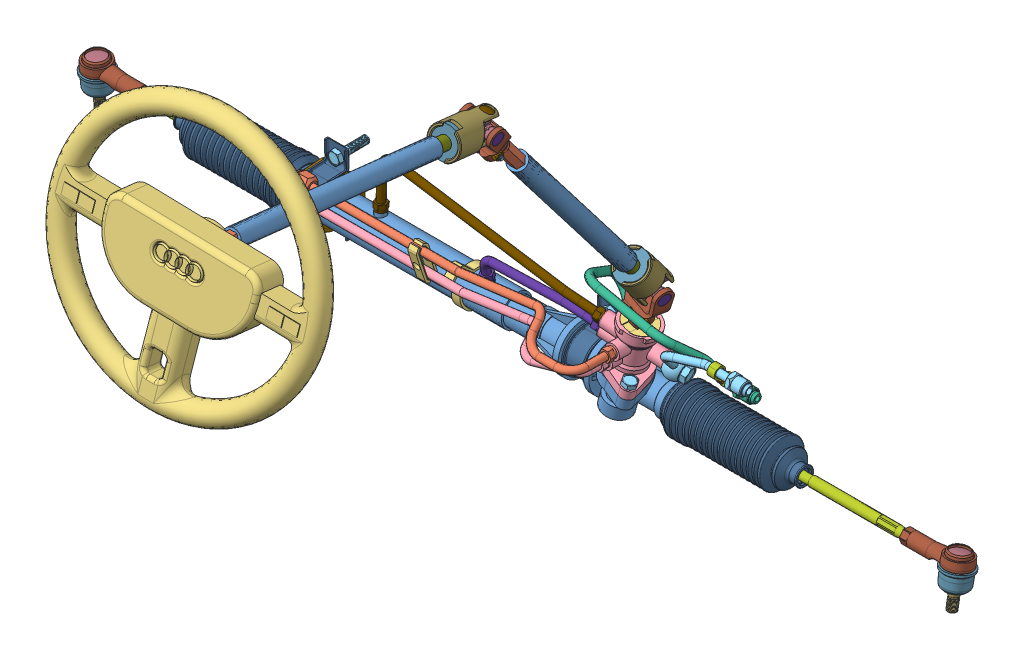
SolidWorks assembly 06, configuration Varsayılan. Lengths in mm.
Overall size (1248.7 876.17 925.76).
101 component instances, 57 part files, 133 mates.
Components (placement in the parent):
- 04-04-1: 04-04 [Varsayılan] at (-125.6681 -6.1583 231.0307) size (234.82 71.44 100.51)
- 04-02-1: 04-02 [Varsayılan] at (194.7465 -6.1583 231.0307) x (0 -1 0) z (-1 0 0) size (38 38 598)
- 04-03-1: 04-03 [Varsayılan] at (38.6922 -33.6461 251.0307) x (0.660997 -0.183782 0.727535) z (-0.700932 0.194939 0.686071) size (25.52 151.51 25.52)
- 04-01-1: 04-01 [Varsayılan] at (50.1654 -6.1583 196.9106) x (0 0 1) z (-1 0 0) size (4.12 38.49 38.49)
- 04-05-1: 04-05 [Varsayılan] at (50.1654 -6.1583 220.9669) x (0 0 1) z (-1 0 0) size (15.7 26.77 26.77)
- 04-06-1: 04-06 [Varsayılan] at (50.1654 -6.1583 203.9669) x (-1 0 0) z (0 0 -1) size (18.46 18.46 19.47)
- 04-07-1: 04-07 [Varsayılan] at (50.1654 -6.1583 223.256) x (0 0 1) z (-1 0 0) size (13.68 21.45 8.13)
- 04-08-1: 04-08 [Varsayılan] at (50.1654 -6.1583 218.4607) x (0 1 0) z (-1 0 0) size (28.57 26.12 28.57)
- 05-14-1: 05-14 [Varsayılan] at (37.0194 -39.6612 251.0307) x (0.963448 -0.267897 0) z (0 0 1) size (30.59 16.59 30.59)
- 05-15-1: 05-15 [Varsayılan] at (41.4642 -23.6793 251.0307) x (0.963434 -0.267944 0) z (0 0 1) size (27.84 7.6 27.84)
- 05-21-1: 05-21 [Varsayılan] at (38.6909 -33.6508 251.0307) x (0.928206 -0.258147 -0.267944) z (0.267944 0.963434 0) size (19.84 10.08 10.35)
- 05-09-1: 05-09 [Varsayılan] at (52.7201 16.7932 251.0307) x (0.963434 -0.267944 0) z (0 0 1) size (31.93 8.54 31.93)
- 05-24-1: 05-24 [Varsayılan] at (55.0081 25.02 251.0307) x (0.963434 -0.267944 0) z (0 0 1) size (34.48 1.46 34.48)
- 05-19-1: 05-19 [Varsayılan] at (66.8414 67.5685 251.0307) x (0.963434 -0.267944 0) z (0 0 1) size (24.62 1.21 24.62)
- 05-10-1: 05-10 [Varsayılan] at (57.7931 35.0339 251.0307) x (0.959223 -0.266824 -0.093253) z (0.089843 -0.024987 0.995642) size (34.48 33.93 34.48)
- 05-11-1: 05-11 [Varsayılan] at (60.4905 44.7327 251.0307) x (0.963421 -0.267991 0) z (0 0 1) size (34.47 2.04 34.47)
- 05-11-2: 05-11 [Varsayılan] at (62.3958 51.5835 251.0307) x (0.963421 -0.267991 0) z (0 0 1) size (34.47 2.04 34.47)
- 05-11-3: 05-11 [Varsayılan] at (64.317 58.4914 251.0307) x (0.963421 -0.267991 0) z (0 0 1) size (34.47 2.04 34.47)
- 05-11-4: 05-11 [Varsayılan] at (66.126 64.9963 251.0307) x (0.963421 -0.267991 0) z (0 0 1) size (34.47 2.04 34.47)
- 05-12-1: 05-12 [Varsayılan] at (67.6163 70.3549 251.0307) x (0.92973 -0.25852 0.26224) z (-0.252651 0.070266 0.965003) size (31.17 6.94 31.17)
- 05-13-1: 05-13 [Varsayılan] at (69.4753 77.0389 251.0307) x (0.963448 -0.267897 0) z (0 0 1) size (29.11 4.72 29.11)
- 05-16-1: 05-16 [Varsayılan] at (67.6164 70.3551 251.0307) x (0.963448 -0.267897 0) z (0 0 1) size (40.01 14.09 40.01)
- 05-22-3: 05-22 [Varsayılan] at (69.4711 77.0238 251.0307) x (0.963434 -0.267944 0) z (0 0 1) size (37.74 2.78 37.74)
- 05-18-1: 05-18 [Varsayılan] at (71.3908 83.9265 251.0307) x (0.96127 -0.267342 0.066993) z (-0.064543 0.01795 0.997753) size (40.8 2.9 40.8)
- 05-25-1: 05-25 [Varsayılan] at (57.2884 33.5525 251.0071) x (0.003637 -0.001047 -0.999993) z (0.963428 -0.267942 0.003784) size (68.03 67.23 77.18)
- formed hex screw_am-1: formed hex screw_am [B18.2.3.2M - Formed hex screw, M10 x 1.5 x 25 --25WS] at (82.3436 33.466 275.1353) x (-0.267944 -0.963434 0) z (0 0 1) size (31.63 18.48 16)
- formed hex screw_am-2: formed hex screw_am [B18.2.3.2M - Formed hex screw, M10 x 1.5 x 25 --25WS] at (36.0727 46.3346 226.9262) x (-0.267944 -0.963434 0) z (0 0 1) size (31.63 18.48 16)
- ROT MİLİ-1: ROT MİLİ [Varsayılan] at (-413.015 77.9473 255.0381) x (1 0 0) z (0 0.086009 -0.996294) size (284.47 41.76 37.89)
  - 02-02-2: 02-02 [Varsayılan] at (3.7615 85.8588 16.6847) size (48.52 36 36)
  - 02-03-3: 02-03 [Varsayılan] at (0.4735 85.8588 16.6847) x (-1 0 0) z (0 0.000479 1) size (257.66 24 24)
  - 02-01-2: 02-01 [Varsayılan] at (2.815 90.0301 15.9062) x (0.295289 -0.871295 0.391981) z (-0.068342 0.389963 0.918291) size (28 21.64 28)
- ROT MİLİ-2: ROT MİLİ [Varsayılan] at (204.5079 -67.283 293.5918) x (-1 0 0) z (0 -0.568825 -0.822459) size (284.47 41.76 37.89)
  - 02-02-2: 02-02 [Varsayılan] at (3.7615 85.8588 16.6847) size (48.52 36 36)
  - 02-03-3: 02-03 [Varsayılan] at (0.4735 85.8588 16.6847) x (-1 0 0) z (0 0.000479 1) size (257.66 24 24)
  - 02-01-2: 02-01 [Varsayılan] at (2.815 90.0301 15.9062) x (0.295289 -0.871295 0.391981) z (-0.068342 0.389963 0.918291) size (28 21.64 28)
- 05-31-1: 05-31 [Varsayılan] at (-390.0863 -6.1583 231.0307) x (0 0.999978 0.006566) z (0 0.006566 -0.999978) size (59.07 38.45 68.81)
- 05-02-1: 05-02 [Varsayılan] at (-409.0863 -6.1583 231.0307) x (-1 0 0) z (0 -0.999688 0.024965) size (174.75 66.11 66.11)
- 05-02-2: 05-02 [Varsayılan] at (105.6183 -6.1583 231.0307) size (174.75 66.11 66.11)
- ROT BAŞI-1: ROT BAŞI [Varsayılan] at (-663.7689 -10.787 321.1728) x (1 0 0) z (0 0.078367 -0.996925) size (99.29 68.51 54.56)
  - 03-01-1: 03-01 [Default] at (-37.7726 9.1069 90.2276) size (90.23 26.88 54.56)
  - 03-02-1: 03-02 [Varsayılan] at (-32.6694 53.6205 89.5242) x (0 -1 0) z (0.136534 0 0.990635) size (58.89 20 20)
  - 03-03-1: 03-03 [Varsayılan] at (-37.7726 -12.3176 90.2276) x (0.135044 0.003215 -0.990834) z (0.99084 0 0.135044) size (26.35 4.4 26.35)
  - 03-04-1: 03-04 [Varsayılan] at (-37.7726 28.686 90.2276) x (0.880691 0 -0.473691) z (0.473691 0 0.880691) size (39.96 25.57 39.96)
  - 03-05-1: 03-05 [Varsayılan] at (-37.7726 -9.866 90.2276) size (25.83 14.98 25.83)
- ROT BAŞI-2: ROT BAŞI [Varsayılan] at (455.2618 -18.6568 141.6394) x (-1 0 0) z (0 0.1653 0.986243) size (99.29 68.51 54.56)
  - 03-01-1: 03-01 [Default] at (-37.7726 9.1069 90.2276) size (90.23 26.88 54.56)
  - 03-02-1: 03-02 [Varsayılan] at (-32.6694 53.6205 89.5242) x (0 -1 0) z (0.136534 0 0.990635) size (58.89 20 20)
  - 03-03-1: 03-03 [Varsayılan] at (-37.7726 -12.3176 90.2276) x (0.135044 0.003215 -0.990834) z (0.99084 0 0.135044) size (26.35 4.4 26.35)
  - 03-04-1: 03-04 [Varsayılan] at (-37.7726 28.686 90.2276) x (0.880691 0 -0.473691) z (0.473691 0 0.880691) size (39.96 25.57 39.96)
  - 03-05-1: 03-05 [Varsayılan] at (-37.7726 -9.866 90.2276) size (25.83 14.98 25.83)
- 05-28-1: 05-28 [Varsayılan] at (-1.0263 -6.1583 231.0307) x (0 -0.759317 -0.650721) z (-1 0 0) size (54.92 54.94 38.56)
- 05-05-3: 05-05 [Varsayılan] at (-153.627 16.7021 236.5228) x (-0.999618 0.007048 -0.026719) z (0.027616 0.221471 -0.974776) size (188.63 111.65 20.5)
- 05-06-2: 05-06 [Varsayılan] at (-308.371 55.2453 229.576) x (-0.999565 0.002273 -0.029406) z (0.029339 -0.025305 -0.999249) size (348.36 140.05 41.18)
- 05-03-3: 05-03 [Varsayılan] at (-414.0863 -6.1583 231.0307) size (295 48.35 43.5)
- 05-33-1: 05-33 [Default] at (-156.8797 44.8002 297.1129) x (-1 0 0) z (0 0.302472 -0.953158) size (421.56 52.06 61.28)
- 05-01-1: 05-01 [Varsayılan] at (-173.5526 -6.1583 231.0307) x (-1 0 0) z (0 0.360562 -0.932735) size (14 137.7 76.92)
- 05-04-1: 05-04 [Varsayılan] at (-390.9146 51.2479 300.523) x (-0.991921 0.112405 0.058801) z (0.000453 0.46666 -0.884437) size (456.96 84.72 60.32)
- 05-08-1: 05-08 [Varsayılan] at (237.637 92.2948 265.4276) x (-0.997325 0.072053 -0.012308) z (-0.043043 -0.714977 -0.697822) size (140.05 46.48 89.04)
- 05-07-1: 05-07 [Varsayılan] at (228.5019 70.3353 246.6946) x (-0.999175 0.040461 0.003581) z (-0.026401 -0.579908 -0.814254) size (231 45.96 100.61)
- formed hex screw_am-3: formed hex screw_am [B18.2.3.2M - Formed hex screw, M12 x 1.75 x 25 --25WS] at (123.6594 37.5337 232.8376) x (-0.948079 0.263674 0.177825) z (-0.177825 -0.903067 0.390959) size (32.76 20.78 18)
- 05-27-1: 05-27 [Varsayılan] at (186.4406 76.9952 250.3773) x (0.044464 0.751851 0.657832) z (0.9987 -0.049876 -0.0105) size (45.68 8 10)
- 05-27-2: 05-27 [Varsayılan] at (196.4276 76.4964 250.2723) x (0.044464 0.751851 0.657832) z (-0.9987 0.049876 0.0105) size (45.68 8 10)
- hex screw_am-2: hex screw_am [B18.6.7M - M5 x 0.8 x 10 Indented HHMS --10S] at (191.9929 87.5632 252.0852) x (-0.024915 -0.657444 0.753091) z (-0.753091 0.507767 0.418362) size (13.8 9.24 8)
- prevailing torque hex nut_am-2: prevailing torque hex nut_am [AM-M5-S] at (191.6665 78.9507 261.9507) x (0.999646 -0.009344 0.024915) z (-0.024915 -0.657444 0.753091) size (8 9.81 5.3)
- 05-29-1: 05-29 [Default] at (-12.3188 -6.1583 205.6444) x (0 1 0) z (0 0 -1) size (108.96 30.28 55.85)
- 05-29-3: 05-29 [Default] at (-390.1285 -6.1115 206.1523) x (0 0.999914 0.013132) z (0 0.013132 -0.999914) size (108.96 30.28 55.85)
- formed hex screw_am-4: formed hex screw_am [B18.2.3.2M - Formed hex screw, M10 x 1.5 x 40 --26WS] at (-390.1268 33.0747 215.2976) x (0 0.013132 -0.999914) z (0.935126 0.354284 0.004653) size (46.63 18.48 16)
- formed hex screw_am-5: formed hex screw_am [B18.2.3.2M - Formed hex screw, M10 x 1.5 x 40 --26WS] at (-390.1268 -45.812 214.2616) x (0 0.013132 -0.999914) z (0.970956 -0.239236 -0.003142) size (46.63 18.48 16)
- formed hex screw_am-6: formed hex screw_am [B18.2.3.2M - Formed hex screw, M10 x 1.5 x 40 --26WS] at (-12.3171 -45.7489 214.2744) x (0 0 -1) z (0.991782 -0.12794 0) size (46.63 18.48 16)
- formed hex screw_am-7: formed hex screw_am [B18.2.3.2M - Formed hex screw, M10 x 1.5 x 40 --26WS] at (-12.3171 33.1445 213.7744) x (0 0 -1) z (0.999706 0.024251 0) size (46.63 18.48 16)
- UNIVERSAL MAFSAL-1: UNIVERSAL MAFSAL [Varsayılan] at (141.0332 165.171 256.4603) x (0.950533 -0.264356 0.163103) z (-0.267944 -0.963434 0) size (48.16 92.97 129.43)
  - 01-01-1: 01-01 [Varsayılan] at (-45.6055 2.036 86.4549) size (47 34.99 57.64)
  - 01-02-1: 01-02 [Varsayılan] at (-45.0363 8.2494 31.8587) x (-0.051046 -0.624854 0.779071) z (0 -0.780088 -0.62567) size (70.3 43.23 43.34)
  - 01-03-1: 01-03 [Varsayılan] at (-51.6055 -0.2661 32.8861) x (1 0 0) z (0 -0.62567 0.780088) size (36 31 16)
  - 01-04-1: 01-04 [Varsayılan] at (-42.5986 38.09 -5.3467) x (-0.998696 0.031938 -0.03982) z (-0.051046 -0.624854 0.779071) size (33.8 41.3 6)
  - 01-05-1: 01-05 [Varsayılan] at (-42.9049 34.3409 -0.6723) x (0.998255 -0.008733 0.058403) z (0.02969 -0.780692 -0.62421) size (32.2 29.4 32.2)
  - 01-06-1: 01-06 [Varsayılan] at (-44.4056 15.9701 22.2324) x (0.051046 0.624854 -0.779071) z (0.993628 0.046715 0.102572) size (75.7 17.29 17.32)
  - 01-07-1: 01-07 [Varsayılan] at (-25.3055 1.2861 40.5406) x (0 0 -1) z (1 0 0) size (16 16 15)
  - 01-08-1: 01-08 [Varsayılan] at (-45.6055 -12.5995 29.4036) x (0.792707 0.38141 -0.475544) z (0 -0.780088 -0.62567) size (16 16 15)
  - 01-07-2: 01-07 [Varsayılan] at (-65.9055 1.2861 40.5406) x (0 -0.633294 0.773912) z (-1 0 0) size (16 16 15)
  - 01-08-2: 01-08 [Varsayılan] at (-45.6055 15.1716 51.6775) x (0.990366 0.086641 -0.108024) z (0 0.780088 0.62567) size (16 16 15)
  - formed hex screw_am-1: formed hex screw_am [B18.2.3.2M - Formed hex screw, M6 x 1.0 x 35 --18WS] at (-62.5055 12.536 76.9549) x (1 0 0) z (0 0.052048 -0.998645) size (39.15 11.55 10)
  - prevailing torque hex nut_am-1: prevailing torque hex nut_am [AM-M6-S] at (-26.1555 12.536 76.9549) x (0 0.889289 0.457347) z (1 0 0) size (10.79 11.55 6.7)
- SHAFT 1-1: SHAFT 1 [Varsayılan] at (102.4 214.0531 312.2723) x (0.979633 -0.04367 -0.195992) z (0.15908 0.764397 0.624813) size (24 24 322.5)
- SHAFT 2-1: SHAFT 2 [Varsayılan] at (126.2619 328.7127 405.9942) x (-0.986743 0.10251 0.125818) z (0.15908 0.764397 0.624813) size (19 19 232)
- UNIVERSAL MAFSAL-2: UNIVERSAL MAFSAL [Varsayılan] at (218.869 550.0843 590.8605) x (0.981176 -0.192592 -0.014194) z (-0.15908 -0.764397 -0.624813) size (48.16 92.97 129.43)
  - 01-01-1: 01-01 [Varsayılan] at (-45.6055 2.036 86.4549) size (47 34.99 57.64)
  - 01-02-1: 01-02 [Varsayılan] at (-45.0363 8.2494 31.8587) x (-0.051046 -0.624854 0.779071) z (0 -0.780088 -0.62567) size (70.3 43.23 43.34)
  - 01-03-1: 01-03 [Varsayılan] at (-51.6055 -0.2661 32.8861) x (1 0 0) z (0 -0.62567 0.780088) size (36 31 16)
  - 01-04-1: 01-04 [Varsayılan] at (-42.5986 38.09 -5.3467) x (-0.998696 0.031938 -0.03982) z (-0.051046 -0.624854 0.779071) size (33.8 41.3 6)
  - 01-05-1: 01-05 [Varsayılan] at (-42.9049 34.3409 -0.6723) x (0.998255 -0.008733 0.058403) z (0.02969 -0.780692 -0.62421) size (32.2 29.4 32.2)
  - 01-06-1: 01-06 [Varsayılan] at (-44.4056 15.9701 22.2324) x (0.051046 0.624854 -0.779071) z (0.993628 0.046715 0.102572) size (75.7 17.29 17.32)
  - 01-07-1: 01-07 [Varsayılan] at (-25.3055 1.2861 40.5406) x (0 0 -1) z (1 0 0) size (16 16 15)
  - 01-08-1: 01-08 [Varsayılan] at (-45.6055 -12.5995 29.4036) x (0.792707 0.38141 -0.475544) z (0 -0.780088 -0.62567) size (16 16 15)
  - 01-07-2: 01-07 [Varsayılan] at (-65.9055 1.2861 40.5406) x (0 -0.633294 0.773912) z (-1 0 0) size (16 16 15)
  - 01-08-2: 01-08 [Varsayılan] at (-45.6055 15.1716 51.6775) x (0.990366 0.086641 -0.108024) z (0 0.780088 0.62567) size (16 16 15)
  - formed hex screw_am-1: formed hex screw_am [B18.2.3.2M - Formed hex screw, M6 x 1.0 x 35 --18WS] at (-62.5055 12.536 76.9549) x (1 0 0) z (0 0.052048 -0.998645) size (39.15 11.55 10)
  - prevailing torque hex nut_am-1: prevailing torque hex nut_am [AM-M6-S] at (-26.1555 12.536 76.9549) x (0 0.889289 0.457347) z (1 0 0) size (10.79 11.55 6.7)
- SHAFT 1-2: SHAFT 1 [Varsayılan] at (178.0086 547.047 663.7863) x (0.966904 0.207955 -0.147823) z (0.105608 0.201209 0.973839) size (24 24 322.5)
- SHAFT 2-2: SHAFT 2 [Varsayılan] at (191.7377 573.2042 790.3853) x (-0.99018 0.111484 0.084346) z (0.105608 0.201209 0.973839) size (19 19 232)
- direksiyon-1: direksiyon [Varsayılan] at (216.7667 620.8908 1021.1848) x (-0.99018 0.111484 0.084346) z (0.105608 0.201209 0.973839) size (350 350 50.57)
Mates (geometry in assembly coordinates):
- Eş Merkezli1: concentric aligned: cylinder of 04-04-1 through (-165.266 -6.1583 231.0307) axis (1 0 0) radius 14; cylinder of 04-02-1 through (-403.2535 -6.1583 231.0307) axis (1 0 0) radius 11.5
- Eş Merkezli2: concentric anti-aligned: cylinder of 04-04-1 through (54.1024 21.7633 251.0307) axis (0.267944 0.963434 0) radius 12.4576; line of 04-03-1 through (79.2895 112.3275 251.0307) axis (-0.267944 -0.963434 0)
- Teğet1: tangent aligned: plane of 04-04-1 through (55.5026 -19.6951 251.0307) normal (-0.267944 -0.963434 0); cone of 04-03-1 through (43.5006 -16.3571 251.0307) axis (-0.267944 -0.963434 0)
- Paralel1: parallel: plane of 04-02-1 through (31.8195 10.9835 238.0307) normal (0 0 1); line of 04-03-1 through (79.2895 112.3275 251.0307) axis (-0.267944 -0.963434 0)
- RackPinionMate1: rack pinion = 20 mm: line of 04-02-1 through (-6.8954 -15.2825 238.0307) axis (-1 0 0); circle of 04-03-1
- Uzaklığı Sınırla1: limit distance = 59.5855 mm anti-aligned: plane of 04-04-1 through (-125.6681 11.3406 231.0307) normal (-1 0 0); plane of 04-02-1 through (-185.2535 -6.1583 250.0307) normal (1 0 0)
- Eş Merkezli3: concentric anti-aligned: cylinder of 04-05-1 through (50.1654 -6.1583 220.9669) axis (0 0 -1) radius 3.705; cylinder of 04-07-1 through (50.1654 -6.1583 223.256) axis (0 0 1) radius 3.7071
- Eş Merkezli4: concentric: sphere of 04-05-1; sphere of 04-07-1
- Eş Merkezli5: concentric anti-aligned: circle of 04-06-1; cylinder of 04-07-1 through (50.1654 -6.1583 223.256) axis (0 0 1) radius 3.7071
- Çakışık1: coincident anti-aligned: plane of 04-05-1 through (59.8031 -6.1583 220.9669) normal (0 0 -1); plane of 04-06-1 through (40.4527 -15.387 220.9669) normal (0 0 1)
- Eş Merkezli6: concentric anti-aligned: circle of 04-06-1; cylinder of 04-08-1 through (50.1654 -6.1583 199.3607) axis (0 0 1) radius 14.285
- Çakışık2: coincident anti-aligned: plane of 04-05-1 through (63.3694 -6.1583 218.4607) normal (0 0 -1); plane of 04-08-1 through (50.1654 -6.1583 218.4607) normal (0 0 1)
- Eş Merkezli7: concentric anti-aligned: cylinder of 04-04-1 through (50.1654 -6.1583 285.0814) axis (0 0 -1) radius 14; cylinder of 04-08-1 through (50.1654 -6.1583 199.3607) axis (0 0 1) radius 14.285
- Çakışık3: coincident anti-aligned: plane of 04-04-1 through (50.1654 -6.1583 201.0307) normal (0 0 -1); circle of 04-08-1
- Eş Merkezli8: concentric anti-aligned: cylinder of 04-04-1 through (50.1654 -6.1583 201.0307) axis (0 0 1) radius 18.85; cylinder of 04-01-1 through (50.1654 -6.1583 196.9106) axis (0 0 -1) radius 13.3852
- Çakışık4: coincident anti-aligned: plane of 04-04-1 through (50.1654 -6.1583 201.0307) normal (0 0 -1); plane of 04-01-1 through (63.5506 -6.1583 201.0307) normal (0 0 1)
- Eş Merkezli9: concentric anti-aligned: cylinder of 04-04-1 through (54.1024 21.7633 251.0307) axis (0.267944 0.963434 0) radius 15.0252; cylinder of 05-15-1 through (43.5005 -16.3572 251.0307) axis (-0.267944 -0.963434 0) radius 13.92
- Çakışık5: coincident anti-aligned: plane of 04-04-1 through (55.5026 -19.6951 251.0307) normal (-0.267944 -0.963434 0); plane of 05-15-1 through (43.5005 -16.3572 251.0307) normal (0.267944 0.963434 0)
- Eş Merkezli10: concentric aligned: cone of 04-03-1 through (38.6923 -33.6459 251.0307) axis (0.267944 0.963434 0); cylinder of 05-21-1 through (38.6909 -33.6508 251.0307) axis (0.267944 0.963434 0) radius 4.26
- Çakışık6: coincident anti-aligned: plane of 05-15-1 through (41.4642 -23.6793 251.0307) normal (-0.267944 -0.963434 0); plane of 05-21-1 through (41.4642 -23.6793 251.0307) normal (0.267944 0.963434 0)
- Eş Merkezli11: concentric aligned: cylinder of 04-04-1 through (54.1024 21.7633 251.0307) axis (0.267944 0.963434 0) radius 15.0252; cone of 05-14-1 through (39.1828 -31.8821 251.0307) axis (0.267944 0.963434 0)
- Teğet2: tangent aligned: cone of 05-14-1 through (41.4644 -23.6786 251.0307) axis (-0.267944 -0.963434 0); plane of 05-15-1 through (41.4642 -23.6793 251.0307) normal (-0.267944 -0.963434 0)
- Çakışık7: coincident: circle of 04-03-1; cone of 05-09-1 through (52.7203 16.7938 251.0307) axis (-0.267944 -0.963434 0)
- Eş Merkezli13: concentric anti-aligned: cylinder of 04-03-1 through (38.6922 -33.6461 251.0307) axis (-0.267944 -0.963434 0) radius 12.7592; cone of 05-24-1 through (55.3984 26.4235 251.0307) axis (0.267944 0.963434 0)
- Çakışık8: coincident aligned: cone of 05-09-1 through (55.008 25.0198 251.0307) axis (-0.267944 -0.963434 0); cone of 05-24-1 through (55.0081 25.02 251.0307) axis (-0.267944 -0.963434 0)
- Eş Merkezli14: concentric anti-aligned: cone of 04-03-1 through (67.1664 68.737 251.0307) axis (0.267944 0.963434 0); circle of 05-19-1
- Teğet4: tangent aligned: cone of 04-03-1 through (66.8415 67.569 251.0307) axis (-0.267944 -0.963434 0); plane of 05-19-1 through (66.8414 67.5685 251.0307) normal (-0.267944 -0.963434 0)
- Eş Merkezli15: concentric anti-aligned: cone of 04-03-1 through (67.1664 68.737 251.0307) axis (0.267944 0.963434 0); cone of 05-10-1 through (58.0414 35.9269 251.0307) axis (-0.267944 -0.963434 0)
- Teğet5: tangent aligned: plane of 05-19-1 through (66.8414 67.5685 251.0307) normal (-0.267944 -0.963434 0); cone of 05-10-1 through (66.8415 67.569 251.0307) axis (-0.267944 -0.963434 0)
- Eş Merkezli17: concentric aligned: cone of 05-10-1 through (60.4905 44.7327 251.0307) axis (0.267944 0.963434 0); cone of 05-11-1 through (61.036 46.6943 251.0307) axis (0.267944 0.963434 0)
- Çakışık10: coincident: circle of 05-10-1; cone of 05-11-1 through (60.4905 44.7327 251.0307) axis (-0.267944 -0.963434 0)
- Eş Merkezli18: concentric aligned: cone of 05-10-1 through (62.3958 51.5835 251.0307) axis (0.267944 0.963434 0); cone of 05-11-2 through (62.9413 53.5452 251.0307) axis (0.267944 0.963434 0)
- Çakışık11: coincident: circle of 05-10-1; cone of 05-11-2 through (62.3958 51.5835 251.0307) axis (-0.267944 -0.963434 0)
- Eş Merkezli19: concentric aligned: cone of 05-10-1 through (64.317 58.4914 251.0307) axis (0.267944 0.963434 0); cone of 05-11-3 through (64.8625 60.4531 251.0307) axis (0.267944 0.963434 0)
- Çakışık12: coincident: circle of 05-10-1; cone of 05-11-3 through (64.317 58.4914 251.0307) axis (-0.267944 -0.963434 0)
- Eş Merkezli20: concentric aligned: cone of 05-10-1 through (66.126 64.9963 251.0307) axis (0.267944 0.963434 0); cone of 05-11-4 through (66.6716 66.9579 251.0307) axis (0.267944 0.963434 0)
- Çakışık13: coincident: circle of 05-10-1; cone of 05-11-4 through (66.126 64.9963 251.0307) axis (-0.267944 -0.963434 0)
- Eş Merkezli22: concentric aligned: cone of 04-03-1 through (67.1664 68.737 251.0307) axis (0.267944 0.963434 0); cone of 05-12-1 through (69.4753 77.0389 251.0307) axis (0.267944 0.963434 0)
- Uzaklık1: distance = 2.73 mm aligned: cone of 05-12-1 through (67.6163 70.3549 251.0307) axis (-0.267944 -0.963434 0); cone of 05-10-1 through (66.8849 67.725 251.0307) axis (-0.267944 -0.963434 0)
- Eş Merkezli23: concentric aligned: cone of 04-03-1 through (67.1664 68.737 251.0307) axis (0.267944 0.963434 0); cone of 05-13-1 through (70.7393 81.5839 251.0307) axis (0.267944 0.963434 0)
- Çakışık14: coincident aligned: cone of 05-12-1 through (69.4753 77.0392 251.0307) axis (-0.267944 -0.963434 0); cone of 05-13-1 through (69.4753 77.0389 251.0307) axis (-0.267944 -0.963434 0)
- Eş Merkezli24: concentric aligned: cone of 05-12-1 through (67.6164 70.3551 251.0307) axis (0.267944 0.963434 0); cone of 05-16-1 through (67.6165 70.3553 251.0307) axis (0.267944 0.963434 0)
- Çakışık15: coincident aligned: cone of 05-12-1 through (67.6163 70.3549 251.0307) axis (-0.267944 -0.963434 0); cone of 05-16-1 through (67.6164 70.3551 251.0307) axis (-0.267944 -0.963434 0)
- Eş Merkezli25: concentric anti-aligned: cone of 05-16-1 through (69.4711 77.0238 251.0307) axis (0.267944 0.963434 0); cylinder of 05-22-3 through (70.216 79.7022 251.0307) axis (-0.267944 -0.963434 0) radius 18.87
- Çakışık16: coincident aligned: circle of 05-16-1; plane of 05-22-3 through (69.4711 77.0238 251.0307) normal (-0.267944 -0.963434 0)
- Eş Merkezli26: concentric anti-aligned: cone of 04-03-1 through (67.1664 68.737 251.0307) axis (0.267944 0.963434 0); cylinder of 05-18-1 through (76.4549 102.1354 251.0307) axis (-0.267944 -0.963434 0) radius 9.8
- Teğet6: tangent aligned: cone of 05-16-1 through (71.391 83.9274 251.0307) axis (-0.267944 -0.963434 0); plane of 05-18-1 through (71.3908 83.9265 251.0307) normal (-0.267944 -0.963434 0)
- Eş Merkezli27: concentric aligned: cylinder of 04-04-1 through (47.6487 -91.2848 275.1353) axis (0.267944 0.963434 0) radius 5.0797; cylinder of 05-25-1 through (77.2955 15.3149 275.1353) axis (0.267944 0.963434 0) radius 4.95
- Eş Merkezli28: concentric aligned: cylinder of 04-04-1 through (1.3778 -78.4162 226.9262) axis (0.267944 0.963434 0) radius 4.95; cylinder of 05-25-1 through (31.0246 28.1834 226.9262) axis (0.267944 0.963434 0) radius 5.0797
- Çakışık17: coincident anti-aligned: plane of 04-04-1 through (81.3463 14.1883 251.0307) normal (0.267944 0.963434 0); plane of 05-25-1 through (54.0168 21.789 251.0071) normal (-0.267944 -0.963434 0)
- Eş Merkezli291: concentric aligned: cylinder of 05-25-1 through (77.2955 15.3149 275.1353) axis (0.267944 0.963434 0) radius 4.95; cylinder of formed hex screw_am-1 through (82.3436 33.466 275.1353) axis (0.267944 0.963434 0) radius 5
- Çakışık181: coincident anti-aligned: plane of 05-25-1 through (57.2884 33.5525 251.0071) normal (0.267944 0.963434 0); plane of formed hex screw_am-1 through (89.4669 24.6032 275.1353) normal (-0.267944 -0.963434 0)
- Eş Merkezli301: concentric aligned: cylinder of 05-25-1 through (31.0246 28.1834 226.9262) axis (0.267944 0.963434 0) radius 5.0797; cylinder of formed hex screw_am-2 through (36.0727 46.3346 226.9262) axis (0.267944 0.963434 0) radius 5
- Çakışık191: coincident anti-aligned: plane of 05-25-1 through (57.2884 33.5525 251.0071) normal (0.267944 0.963434 0); plane of formed hex screw_am-2 through (43.196 37.4718 226.9262) normal (-0.267944 -0.963434 0)
- Eş Merkezli32: concentric anti-aligned: cylinder of 04-02-1 through (-403.2535 -6.1583 231.0307) axis (1 0 0) radius 11.5; cylinder of ROT MİLİ-1/02-02-2 through (-409.407 -6.1583 231.0307) axis (-1 0 0) radius 18
- Çakışık20: coincident anti-aligned: plane of 04-02-1 through (-403.2535 -6.1583 231.0307) normal (-1 0 0); plane of ROT MİLİ-1/02-02-2 through (-403.2535 -6.1583 231.0307) normal (1 0 0)
- Eş Merkezli33: concentric aligned: cylinder of 04-02-1 through (-403.2535 -6.1583 231.0307) axis (1 0 0) radius 11.5; cylinder of ROT MİLİ-2/02-02-2 through (200.8999 -6.1583 231.0307) axis (1 0 0) radius 18
- Çakışık21: coincident anti-aligned: plane of 04-02-1 through (194.7465 -6.1583 231.0307) normal (1 0 0); plane of ROT MİLİ-2/02-02-2 through (194.7465 -6.1583 231.0307) normal (-1 0 0)
- Eş Merkezli36: concentric anti-aligned: cylinder of 04-02-1 through (-403.2535 -6.1583 231.0307) axis (1 0 0) radius 11.5; cylinder of 05-02-2 through (105.6183 -6.1583 231.0307) axis (-1 0 0) radius 11.6806
- Çakışık23: coincident anti-aligned: plane of 04-04-1 through (105.6183 12.6764 231.0307) normal (1 0 0); plane of 05-02-2 through (105.6183 19.7754 231.0307) normal (-1 0 0)
- Eş Merkezli37: concentric aligned: cylinder of ROT MİLİ-1/02-03-3 through (-423.5415 -6.1583 231.0307) axis (1 0 0) radius 5.0675; cylinder of ROT BAŞI-1/03-01-1 through (-666.2915 -6.1583 231.0307) axis (1 0 0) radius 9.5
- Çakışık24: coincident aligned: circle of ROT MİLİ-1/02-03-3; plane of ROT BAŞI-1/03-01-1 through (-629.5415 3.069 222.1124) normal (1 0 0)
- Eş Merkezli38: concentric aligned: cylinder of ROT MİLİ-2/02-03-3 through (215.0344 -6.1583 231.0307) axis (-1 0 0) radius 6.5; cylinder of ROT BAŞI-2/03-01-1 through (457.7844 -6.1583 231.0307) axis (-1 0 0) radius 9.5
- Çakışık25: coincident aligned: circle of ROT MİLİ-2/02-03-3; plane of ROT BAŞI-2/03-01-1 through (421.0344 3.8139 239.1074) normal (-1 0 0)
- Eş Merkezli39: concentric anti-aligned: cylinder of 04-04-1 through (-125.6681 -6.1583 231.0307) axis (-1 0 0) radius 21.75; cylinder of 05-28-1 through (-23.5863 -6.1583 231.0307) axis (1 0 0) radius 25.75
- Çakışık26: coincident anti-aligned: plane of 04-04-1 through (6.9737 26.3417 231.0307) normal (-1 0 0); plane of 05-28-1 through (6.9737 -6.1583 231.0307) normal (1 0 0)
- Eş Merkezli304: concentric anti-aligned: cylinder of 05-25-1 through (101.3768 36.6462 241.4658) axis (-0.949417 0.264046 0.169963) radius 5; cylinder of 05-05-3 through (21.6687 58.8141 255.7351) axis (0.949417 -0.264046 -0.169963) radius 7
- Çakışık194: coincident anti-aligned: plane of 05-25-1 through (21.5918 48.3269 253.9468) normal (-0.949417 0.264046 0.169963); plane of 05-05-3 through (26.0012 62.678 256.2827) normal (0.949417 -0.264046 -0.169963)
- Eş Merkezli305: concentric anti-aligned: cylinder of 05-25-1 through (105.7565 50.9201 243.7559) axis (-0.949417 0.264046 0.169963) radius 5; cylinder of 05-06-2 through (26.0484 73.088 258.0251) axis (0.949417 -0.264046 -0.169963) radius 7
- Çakışık195: coincident anti-aligned: plane of 05-25-1 through (21.5918 48.3269 253.9468) normal (-0.949417 0.264046 0.169963); plane of 05-06-2 through (30.1982 77.1184 257.2936) normal (0.949417 -0.264046 -0.169963)
- Eş Merkezli306: concentric anti-aligned: cylinder of 04-02-1 through (-403.2535 -6.1583 231.0307) axis (1 0 0) radius 11.5; cylinder of 05-03-3 through (-119.0863 -6.1583 231.0307) axis (-1 0 0) radius 21.75
- Çakışık196: coincident anti-aligned: plane of 04-04-1 through (-119.0863 12.8417 231.0307) normal (-1 0 0); plane of 05-03-3 through (-119.0863 -6.1583 231.0307) normal (1 0 0)
- Eş Merkezli307: concentric anti-aligned: cylinder of 05-31-1 through (-405.0863 -6.1583 231.0307) axis (1 0 0) radius 20.7084; cylinder of 05-03-3 through (-119.0863 -6.1583 231.0307) axis (-1 0 0) radius 21.75
- Eş Merkezli308: concentric anti-aligned: cylinder of 05-02-1 through (-409.0863 -6.1583 231.0307) axis (1 0 0) radius 25.6827; cylinder of 05-03-3 through (-119.0863 -6.1583 231.0307) axis (-1 0 0) radius 21.75
- Uzaklık2: distance = 5 mm aligned: plane of 05-03-3 through (-414.0863 -6.1583 231.0307) normal (-1 0 0); plane of 05-31-1 through (-409.0863 -6.1583 231.0307) normal (-1 0 0)
- Çakışık197: coincident anti-aligned: plane of 05-31-1 through (-409.0863 -6.1583 231.0307) normal (-1 0 0); plane of 05-02-1 through (-409.0863 -6.8058 205.105) normal (1 0 0)
- Kilitle1: lock: unknown of 05-05-3; unknown of 05-03-3
- Kilitle2: lock: unknown of 05-06-2; unknown of 05-03-3
- Eş Merkezli309: concentric anti-aligned: cylinder of 05-25-1 through (65.5394 62.2675 263.2963) axis (-0.003655 0.006527 0.999972) radius 5; cylinder of 05-33-1 through (65.3201 62.6591 323.2946) axis (0.003655 -0.006527 -0.999972) radius 4
- Çakışık198: coincident anti-aligned: plane of 05-25-1 through (60.6154 54.5186 283.3295) normal (-0.003655 0.006527 0.999972); plane of 05-33-1 through (65.4663 62.3981 283.2958) normal (0.003655 -0.006527 -0.999972)
- Eş Merkezli310: concentric anti-aligned: cylinder of 05-03-3 through (-119.0863 -6.1583 231.0307) axis (-1 0 0) radius 21.75; cylinder of 05-01-1 through (-185.5526 -6.1583 231.0307) axis (1 0 0) radius 21.7671
- Teğet7: tangent anti-aligned: cylinder of 05-33-1 through (-125.1716 75.9211 306.9887) axis (-1 0 0) radius 5; plane of 05-01-1 through (-172.5526 79.1244 302.774) normal (0 -0.309917 0.950763)
- Eş Merkezli312: concentric anti-aligned: cylinder of 05-25-1 through (55.8376 46.5086 263.3637) axis (-0.003655 0.006527 0.999972) radius 5; circle of 05-04-1
- Çakışık201: coincident anti-aligned: plane of 05-25-1 through (60.6154 54.5186 283.3295) normal (-0.003655 0.006527 0.999972); plane of 05-04-1 through (60.0822 49.1995 283.3622) normal (0.003655 -0.006527 -0.999972)
- Kilitle3: lock: unknown of 05-01-1; unknown of 05-04-1
- Eş Merkezli313: concentric aligned: cylinder of 05-25-1 through (18.9204 66.663 252.4828) axis (0.948079 -0.263674 -0.177825) radius 5; cylinder of 05-08-1 through (83.9328 48.5821 240.2888) axis (0.948079 -0.263674 -0.177825) radius 5
- Çakışık202: coincident anti-aligned: plane of 05-25-1 through (97.3407 44.8532 237.774) normal (0.948079 -0.263674 -0.177825); plane of 05-08-1 through (101.3663 42.9237 262.0976) normal (-0.948079 0.263674 0.177825)
- Eş Merkezli314: concentric anti-aligned: cylinder of 05-25-1 through (91.8203 46.3885 292.2446) axis (-0.66663 0.185399 -0.721963) radius 5; cylinder of 05-07-1 through (28.8333 63.9061 224.0295) axis (0.66663 -0.185399 0.721963) radius 3
- Çakışık203: coincident anti-aligned: plane of 05-25-1 through (40.3095 60.7144 222.006) normal (-0.66663 0.185399 -0.721963); plane of 05-07-1 through (29.8159 63.3842 232.381) normal (0.66663 -0.185399 0.721963)
- Eş Merkezli3151: concentric aligned: cylinder of 05-08-1 through (83.9328 48.5821 240.2888) axis (0.948079 -0.263674 -0.177825) radius 5; cylinder of formed hex screw_am-3 through (123.6594 37.5337 232.8376) axis (0.948079 -0.263674 -0.177825) radius 6
- Çakışık2041: coincident anti-aligned: plane of 05-08-1 through (120.4882 37.9933 258.8874) normal (0.948079 -0.263674 -0.177825); plane of formed hex screw_am-3 through (113.5621 36.0564 224.8326) normal (-0.948079 0.263674 0.177825)
- Eş Merkezli316: concentric anti-aligned: cylinder of 05-08-1 through (180.9639 95.1251 266.0234) axis (0.9987 -0.049876 -0.0105) radius 5; cylinder of 05-27-1 through (197.4805 94.3003 265.8497) axis (-0.9987 0.049876 0.0105) radius 8
- Kilitle4: lock: unknown of 05-07-1; unknown of 05-27-1
- Eş Merkezli320: concentric anti-aligned: cylinder of 05-27-1 through (191.5494 75.8607 265.4902) axis (0.024915 0.657444 -0.753091) radius 2.5; cylinder of 05-27-2 through (192.1473 91.6394 247.416) axis (-0.024915 -0.657444 0.753091) radius 2.5
- Çakışık206: coincident anti-aligned: plane of 05-27-1 through (196.4276 76.4964 250.2723) normal (0.024915 0.657444 -0.753091); plane of 05-27-2 through (186.4406 76.9952 250.3773) normal (-0.024915 -0.657444 0.753091)
- Paralel2: parallel aligned: plane of 05-27-1 through (196.1608 71.9853 246.3253) normal (0.9987 -0.049876 -0.0105); plane of 05-27-2 through (196.1608 71.9853 246.3253) normal (0.9987 -0.049876 -0.0105)
- Eş Merkezli3221: concentric anti-aligned: cylinder of 05-27-2 through (192.1473 91.6394 247.416) axis (-0.024915 -0.657444 0.753091) radius 2.5; cylinder of hex screw_am-2 through (192.6257 104.2623 232.9567) axis (0.024915 0.657444 -0.753091) radius 2.5
- Çakışık2091: coincident anti-aligned: plane of 05-27-2 through (187.1989 90.2901 259.353) normal (0.024915 0.657444 -0.753091); plane of hex screw_am-2 through (193.5418 86.4567 256.2164) normal (-0.024915 -0.657444 0.753091)
- Eş Merkezli3231: concentric anti-aligned: cylinder of 05-27-1 through (191.5494 75.8607 265.4902) axis (0.024915 0.657444 -0.753091) radius 2.5; cylinder of prevailing torque hex nut_am-2 through (192.2903 95.4115 243.0952) axis (-0.024915 -0.657444 0.753091) radius 2.5
- Çakışık2101: coincident anti-aligned: plane of 05-27-1 through (197.0863 87.1616 262.2604) normal (-0.024915 -0.657444 0.753091); plane of prevailing torque hex nut_am-2 through (191.7554 85.9152 260.9959) normal (0.024915 0.657444 -0.753091)
- Eş Merkezli324: concentric anti-aligned: cylinder of 05-28-1 through (-23.5863 -6.1583 231.0307) axis (1 0 0) radius 25.75; circle of 05-29-1
- Paralel3: parallel aligned: plane of 04-08-1 through (50.1654 -6.1583 192.3407) normal (0 0 -1); plane of 05-29-1 through (-34.6242 -64.6442 206.6444) normal (0 0 -1)
- Kilitle5: lock: unknown of 05-28-1; unknown of 05-29-1
- Paralel4: parallel aligned: plane of 05-31-1 through (-371.0863 -17.9763 189.9514) normal (0 0 -1); plane of 05-29-1 through (-34.6242 -64.6442 206.6444) normal (0 0 -1)
- Eş Merkezli3233: concentric anti-aligned: cylinder of 05-31-1 through (-405.0863 -6.4449 231.5364) axis (1 0 0) radius 24.365; circle of 05-29-3
- Paralel6: parallel aligned: plane of 05-31-1 through (-409.0863 5.4203 190.105) normal (0 0.013132 -0.999914); plane of 05-29-3 through (-412.4339 -64.6054 206.3842) normal (0 0.013132 -0.999914)
- Kilitle6: lock: unknown of 05-31-1; unknown of 05-29-3
- Eş Merkezli3234: concentric anti-aligned: circle of 05-29-3; cylinder of formed hex screw_am-4 through (-390.1268 33.0747 215.2976) axis (0 -0.013132 0.999914) radius 5
- Uzaklık3: distance = 1 mm aligned: plane of formed hex screw_am-4 through (-393.3999 41.7993 208.7816) normal (0 0.013132 -0.999914); plane of 05-29-3 through (-412.4339 -64.6054 206.3842) normal (0 0.013132 -0.999914)
- Eş Merkezli32351: concentric aligned: cylinder of 05-29-3 through (-390.1268 -45.5805 196.6331) axis (0 -0.013132 0.999914) radius 6.75; cylinder of formed hex screw_am-5 through (-390.1268 -45.812 214.2616) axis (0 -0.013132 0.999914) radius 5
- Çakışık21041: coincident anti-aligned: plane of 05-29-3 through (-402.1268 -39.2149 207.7177) normal (0 -0.013132 0.999914); plane of formed hex screw_am-5 through (-387.9167 -36.7564 207.75) normal (0 0.013132 -0.999914)
- Eş Merkezli3236: concentric anti-aligned: circle of 05-29-1; cylinder of formed hex screw_am-6 through (-12.3171 -45.7489 214.2744) axis (0 0 1) radius 5
- Çakışık2105: coincident anti-aligned: plane of 05-29-1 through (-24.3171 -39.2383 207.6444) normal (0 0 1); plane of formed hex screw_am-6 through (-11.1352 -36.5872 207.6444) normal (0 0 -1)
- Eş Merkezli3237: concentric anti-aligned: circle of 05-29-1; cylinder of formed hex screw_am-7 through (-12.3171 33.1445 213.7744) axis (0 0 1) radius 5
- Uzaklık4: distance = 0.5 mm aligned: plane of 05-29-1 through (-34.6242 -64.6442 206.6444) normal (0 0 -1); plane of formed hex screw_am-7 through (-12.5411 42.3794 207.1444) normal (0 0 -1)
- Eş Merkezli3238: concentric aligned: line of 04-03-1 through (79.2895 112.3275 251.0307) axis (-0.267944 -0.963434 0); circle of UNIVERSAL MAFSAL-1/01-01-1
- Çakışık2106: coincident aligned: circle of 04-03-1; plane of UNIVERSAL MAFSAL-1/01-01-1 through (56.952 118.54 247.1978) normal (-0.267944 -0.963434 0)
- Eş Merkezli32352: concentric anti-aligned: cylinder of UNIVERSAL MAFSAL-1/01-06-1 through (90.3576 156.1883 264.974) axis (-0.15908 -0.764397 -0.624813) radius 8.5; circle of SHAFT 1-1
- Çakışık21042: coincident aligned: plane of UNIVERSAL MAFSAL-1/01-06-1 through (101.6217 200.7615 292.7206) normal (-0.15908 -0.764397 -0.624813); plane of SHAFT 1-1 through (98.8207 196.8542 298.214) normal (-0.15908 -0.764397 -0.624813)
- Paralel7: parallel anti-aligned: line of UNIVERSAL MAFSAL-1/01-06-1 through (96.6384 201.8797 292.6214) axis (0.829203 -0.446936 0.335664); line of SHAFT 1-1 through (97.0771 201.6432 292.799) axis (-0.829203 0.446936 -0.335664)
- Eş Merkezli32353: concentric aligned: cylinder of SHAFT 1-1 through (150.1239 443.3722 499.7161) axis (-0.15908 -0.764397 -0.624813) radius 12; cylinder of SHAFT 2-1 through (158.8733 485.414 534.0808) axis (-0.15908 -0.764397 -0.624813) radius 9.5
- Paralel8: parallel aligned: plane of SHAFT 1-1 through (154.9384 437.8064 505.2996) normal (-0.870607 0.407048 -0.276324); plane of SHAFT 2-1 through (153.2633 487.1579 525.3733) normal (-0.870607 0.407048 -0.276324)
- Uzaklık5: distance = 50 mm anti-aligned: plane of SHAFT 1-1 through (150.1239 443.3722 499.7161) normal (0.15908 0.764397 0.624813); plane of SHAFT 2-1 through (158.0779 481.592 530.9568) normal (-0.15908 -0.764397 -0.624813)
- Eş Merkezli32354: concentric aligned: cylinder of SHAFT 2-1 through (158.8733 485.414 534.0808) axis (-0.15908 -0.764397 -0.624813) radius 9.5; circle of UNIVERSAL MAFSAL-2/01-01-1
- Çakışık21046: coincident aligned: circle of SHAFT 2-1; plane of UNIVERSAL MAFSAL-2/01-01-1 through (140.1107 510.5784 551.2841) normal (-0.15908 -0.764397 -0.624813)
- Eş Merkezli32355: concentric aligned: cylinder of UNIVERSAL MAFSAL-2/01-06-1 through (170.0141 531.8155 590.0667) axis (-0.105608 -0.201209 -0.973839) radius 8.5; cylinder of SHAFT 1-2 through (209.691 607.4098 955.9379) axis (-0.105608 -0.201209 -0.973839) radius 12
- Çakışık21047: coincident aligned: plane of UNIVERSAL MAFSAL-2/01-06-1 through (177.6933 549.3304 640.2443) normal (-0.105608 -0.201209 -0.973839); plane of SHAFT 1-2 through (175.6324 542.5198 641.8749) normal (-0.105608 -0.201209 -0.973839)
- Paralel9: parallel anti-aligned: line of UNIVERSAL MAFSAL-2/01-06-1 through (175.2552 550.1861 640.3319) axis (0.684593 -0.724999 0.075555); line of SHAFT 1-2 through (175.6174 549.8025 640.3719) axis (-0.684593 0.724999 -0.075555)
- Eş Merkezli32356: concentric aligned: cylinder of SHAFT 1-2 through (209.691 607.4098 955.9379) axis (-0.105608 -0.201209 -0.973839) radius 12; cylinder of SHAFT 2-2 through (213.3873 614.4522 990.0223) axis (-0.105608 -0.201209 -0.973839) radius 9.5
- Uzaklık6: distance = 30 mm anti-aligned: plane of SHAFT 2-2 through (212.8592 613.4461 985.1531) normal (-0.105608 -0.201209 -0.973839); plane of SHAFT 1-2 through (209.691 607.4098 955.9379) normal (0.105608 0.201209 0.973839)
- Eş Merkezli32357: concentric anti-aligned: cylinder of SHAFT 1-2 through (209.691 607.4098 955.9379) axis (-0.105608 -0.201209 -0.973839) radius 12; cylinder of direksiyon-1 through (213.5985 614.8545 991.9696) axis (0.105608 0.201209 0.973839) radius 32.5
- Paralel10: parallel anti-aligned: plane of SHAFT 2-2 through (216.4096 612.6007 1017.8024) normal (-0.091596 -0.973184 0.211007); plane of direksiyon-1 through (214.7146 612.7915 1017.9464) normal (0.091596 0.973184 -0.211007)
- Çakışık21050: coincident aligned: circle of SHAFT 2-2; plane of direksiyon-1 through (223.6677 617.7256 1015.956) normal (-0.105608 -0.201209 -0.973839)
